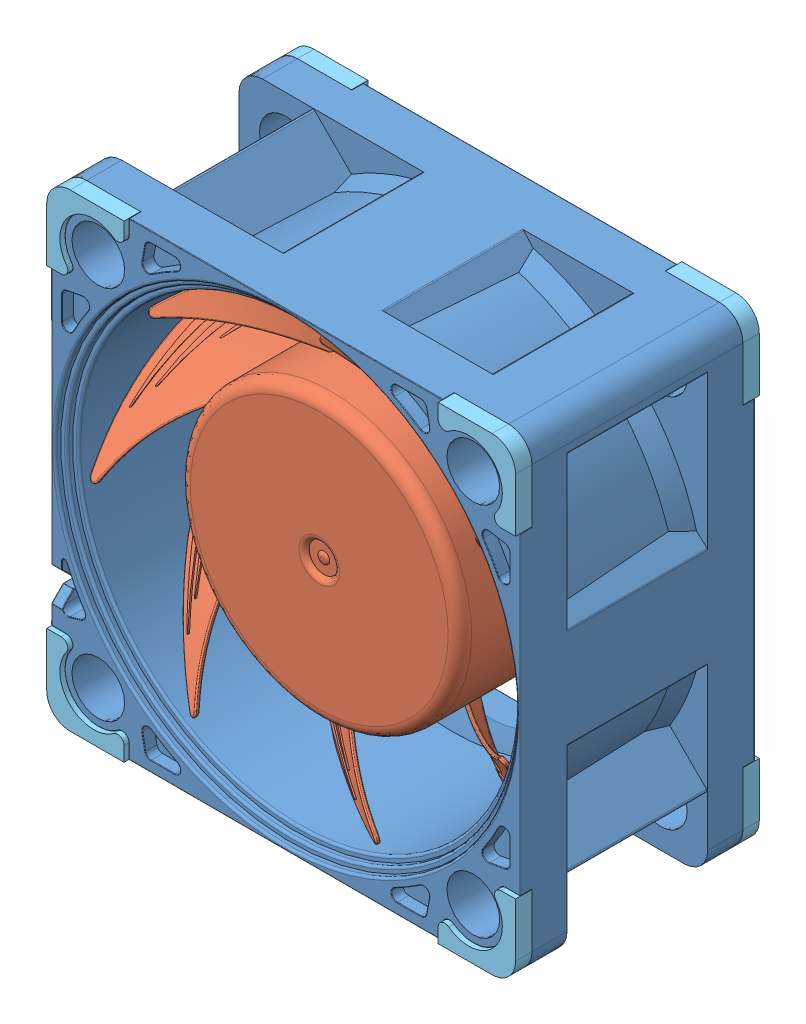
SolidWorks assembly NF-A4x20, configuration Predeterminado. Lengths in mm.
Overall size (49.24 49.24 20.8).
33 component instances, 18 part files, 22 mates.
Components (placement in the parent):
- Case20-1: Case20 [Predeterminado] at origin size (40 40 20.31)
- Impeller20-1: Impeller20 [Predeterminado] at (0 0 5.65) x (-0.910833 -0.412774 0) z (0 0 1) size (37.2 37.2 13.1)
- Magnet 20-1: Magnet 20 [Predeterminado] at (0 0 0.35) size (2 2 1.8)
- Back plate 20-1: Back plate 20 [Predeterminado] at (0 0 -0.05) size (19.4 19.4 0.4)
- Silent block-1: Silent block [Predeterminado] at (-16 16 -0.4) size (6.6 6.6 1.4)
- Silent block-2: Silent block [Predeterminado] at (-16 16 19) size (6.6 6.6 1.4)
- Silent block-3: Silent block [Predeterminado] at (16 16 -0.4) x (0 -1 0) z (0 0 1) size (6.6 6.6 1.4)
- Silent block-4: Silent block [Predeterminado] at (16 -16 -0.4) x (-1 0 0) z (0 0 1) size (6.6 6.6 1.4)
- Silent block-5: Silent block [Predeterminado] at (-16 -16 -0.4) x (0 1 0) z (0 0 1) size (6.6 6.6 1.4)
- Silent block-6: Silent block [Predeterminado] at (16 16 19) x (0 -1 0) z (0 0 1) size (6.6 6.6 1.4)
- Silent block-7: Silent block [Predeterminado] at (16 -16 19) x (-1 0 0) z (0 0 1) size (6.6 6.6 1.4)
- Silent block-8: Silent block [Predeterminado] at (-16 -16 19) x (0 1 0) z (0 0 1) size (6.6 6.6 1.4)
- Brushless motor-1: Brushless motor [Predeterminado] at (0 0 4) x (0.568712 -0.822537 0) z (0 0 1) size (16 16 8.48)
  - Board-1: Board [Predeterminado] at origin size (16 16 0.8)
  - Stator-1: Stator [Predeterminado] at (0 0 3.55) size (11.93 12 5.5)
  - Hall Effect sensor-1: Hall Effect sensor [WE] at (-5.3023 -0.9391 0) x (-0.233503 0.972356 0) z (-0.972356 -0.233503 0) size (6.3 1.6 2.6)
  - Controller-1: Controller [Predeterminado] at (5.1574 2.3195 0) x (0.319288 -0.947658 0) z (0.947658 0.319288 0) size (4.81 0.99 3)
  - Coil-1: Coil [Predeterminado] at (0 -5.01 1.29) x (-1 0 0) z (0 1 0) size (2.38 5.38 1.58)
  - Coil-2: Coil [Predeterminado] at (-4.3388 -2.505 1.29) x (-0.5 0.866025 0) z (0.866025 0.5 0) size (2.38 5.38 1.58)
  - Coil-3: Coil [Predeterminado] at (-4.3388 2.505 1.29) x (0.5 0.866025 0) z (0.866025 -0.5 0) size (2.38 5.38 1.58)
  - Coil-4: Coil [Predeterminado] at (0 5.01 1.29) x (1 0 0) z (0 -1 0) size (2.38 5.38 1.58)
  - Coil-5: Coil [Predeterminado] at (4.3388 2.505 1.29) x (0.5 -0.866025 0) z (-0.866025 -0.5 0) size (2.38 5.38 1.58)
  - Coil-6: Coil [Predeterminado] at (4.3388 -2.505 1.29) x (-0.5 -0.866025 0) z (-0.866025 0.5 0) size (2.38 5.38 1.58)
  - Pieza2^Brushless motor-1: Pieza2^Brushless motor [Predeterminado] at origin size (10.72 12.51 6.88) (virtual)
  - Pieza3^Brushless motor-1: Pieza3^Brushless motor [Predeterminado] at (0 0 0.8) size (4.1 0.74 1.7) (virtual)
- Shaft-1: Shaft [Predeterminado] at (0 0 16.35) x (0.952278 -0.305233 0) z (0 0 1) (suppressed, hidden)
- Oil Bearing-1: Oil Bearing [Predeterminado] at (0 0 4) x (0.568712 -0.822537 0) z (0 0 -1) size (5 5 5)
  - Bearing-1: Bearing [Predeterminado] at origin size (5 5 5)
  - Bearing gasket-1: Bearing gasket [Predeterminado] at (0 0 -1.3) size (2 2 0.5)
  - Oil-1: Oil [Predeterminado] at (0 0 -4.5) size (4 4 2.7)
  - Bearing gasket-2: Bearing gasket [Predeterminado] at (0 0 -4.5) size (2 2 0.5)
- Rotor-1: Rotor [Predeterminado] at (0 0 5.65) x (0.792012 -0.610506 0) z (0 0 -1) size (16.45 16.45 6.1)
- Magnetic screen-1: Magnetic screen [Predeterminado] at (0 0 5.65) size (16.85 16.85 6)
Mates (geometry in assembly coordinates):
- Coincidente1: coincident aligned: plane of Case20-1 through (0 0 0) normal (0 0 1)
- Coincidente2: coincident aligned: plane of Case20-1 through (0 0 0) normal (0 1 0)
- Coincidente3: coincident aligned: plane of Case20-1 through (0 0 0) normal (1 0 0)
- Concéntrica1: concentric aligned: cylinder of Case20-1 through (0 0 2) axis (0 0 -1) radius 12; cylinder of Impeller20-1 through (0 0 17.15) axis (0 0 -1) radius 12
- Distancia1: distance = 2.85 mm aligned: plane of Impeller20-1 through (0 0 17.15) normal (0 0 1); plane of Case20-1 through (-18.7563 13.9563 20) normal (0 0 1)
- Coincidente4: coincident anti-aligned: plane of Case20-1 through (0 0 2.15) normal (0 0 -1); plane of Magnet-1 through (0 0 2.15) normal (0 0 1)
- Concéntrica2: concentric aligned: cylinder of Case20-1 through (0 0 2.15) axis (0 0 -1) radius 1; cylinder of Magnet-1 through (0 0 2.15) axis (0 0 -1) radius 1
- Concéntrica3: concentric aligned: cylinder of Case20-1 through (0 0 0.35) axis (0 0 -1) radius 9.95; cylinder of Back plate-1 through (0 0 0.35) axis (0 0 -1) radius 9.7
- Coincidente5: coincident anti-aligned: plane of Case20-1 through (0 0 0.35) normal (0 0 -1); plane of Back plate-1 through (0 0 0.35) normal (0 0 1)
- Coincidente6: coincident anti-aligned: plane of Case20-1 through (-18 18 1) normal (0 0 -1); plane of Silent block-1 through (-18.7563 13.9563 1) normal (0 0 1)
- Coincidente7: coincident anti-aligned: plane of Case20-1 through (-13.4 0 1) normal (-1 0 0); plane of Silent block-1 through (-13.4 20 1) normal (1 0 0)
- Coincidente8: coincident anti-aligned: plane of Case20-1 through (0 13.4 1) normal (0 1 0); plane of Silent block-1 through (-20 13.4 1) normal (0 -1 0)
- Concéntrica4: concentric aligned: cylinder of Case20-1 through (0 0 2) axis (0 0 -1) radius 12; cylinder of Brushless motor-1/Board-1 through (0 0 4.8) axis (0 0 -1) radius 8
- Concéntrica5: concentric aligned: circle of Impeller20-1; circle of Shaft-1
- Coincidente9: coincident anti-aligned: plane of Impeller20-1 through (0 0 16.35) normal (0 0 -1); plane of Shaft-1 through (0 0 16.35) normal (0 0 1)
- Concéntrica6: concentric aligned: cylinder of Brushless motor-1/Stator-1 through (0 0 10.3) axis (0 0 -1) radius 2.5; cylinder of Oil Bearing-1/Bearing-1 through (0 0 4) axis (0 0 -1) radius 2.5
- Coincidente10: coincident aligned: plane of Brushless motor-1/Board-1 through (0 0 4) normal (0 0 -1); plane of Oil Bearing-1/Bearing-1 through (-0.8531 1.2338 4) normal (0 0 -1)
- Distancia2: distance = 1.5 mm anti-aligned: plane of Case20-1 through (0 0 2.5) normal (0 0 1); plane of Brushless motor-1/Board-1 through (0 0 4) normal (0 0 -1)
- Concéntrica7: concentric aligned: cylinder of Impeller20-1 through (0 0 17.152) axis (0 0 -1) radius 8.425; cylinder of Rotor-1 through (0 0 11.75) axis (0 0 -1) radius 8.225
- Coincidente11: coincident aligned: plane of Impeller20-1 through (0 0 5.65) normal (0 0 -1); plane of Rotor-1 through (0 0 5.65) normal (0 0 -1)
- Coincidente12: coincident aligned: plane of Impeller20-1 through (0 0 5.65) normal (0 0 -1); plane of Magnetic screen-1 through (0 0 5.65) normal (0 0 -1)
- Concéntrica8: concentric aligned: cylinder of Rotor-1 through (0 0 11.75) axis (0 0 -1) radius 8.225; cylinder of Magnetic screen-1 through (0 0 11.65) axis (0 0 -1) radius 8.425
